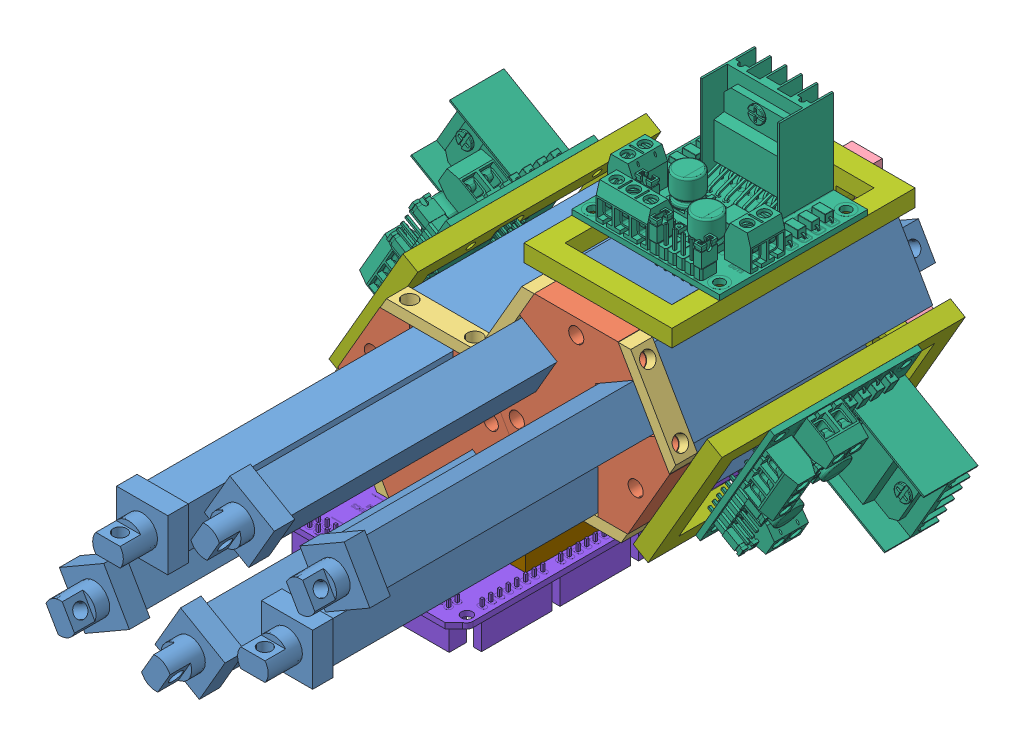
SolidWorks assembly DeltaArray, configuration Default. Lengths in mm.
Overall size (160.54 122.18 184.94).
31 component instances, 9 part files, 18 mates.
Components (placement in the parent):
- Delta_Module-1: Delta_Module [Default] at (-24.2565 17.4629 11.2137) size (68.32 71 180)
  - 3inLinearActuator-1: 3inLinearActuator [Default] at (52.9296 100.0903 59.6287) size (23 19 180)
  - 3inLinearActuator-2: 3inLinearActuator [Default] at (66.3243 77.8201 59.6287) x (-0.5 -0.866025 0) z (0 0 1) size (23 19 180)
  - 3inLinearActuator-3: 3inLinearActuator [Default] at (40.3403 77.3551 59.6287) x (-0.5 0.866025 0) z (0 0 1) size (23 19 180)
  - Connector-1: Connector [Default] at (53.1981 85.0885 129.6287) x (-0.5 0.866025 0) z (0.866025 0.5 0) size (54.66 6.35 47.33)
  - Edge_Piece-1: Edge_Piece [Default] at (53.1981 107.9385 129.6287) x (-1 0 0) z (0 0 1) size (29.97 3.17 6.35)
  - Edge_Piece-2: Edge_Piece [Default] at (33.4094 73.6635 129.6287) x (0.5 -0.866025 0) z (0 0 1) size (29.97 3.17 6.35)
  - Edge_Piece-3: Edge_Piece [Default] at (72.9867 73.6635 129.6287) x (0.5 0.866025 0) z (0 0 1) size (29.97 3.17 6.35)
  - BottomConnector-1: BottomConnector [Default] at (53.1981 85.0885 58.4387) x (0.5 -0.866025 0) z (0.866025 0.5 0) size (46.87 7.62 40.59)
- Delta_Module-2: Delta_Module [Default] at (118.44 38.4209 11.2137) x (0.5 0.866025 0) z (0 0 1) size (68.32 71 180)
  - 3inLinearActuator-1: 3inLinearActuator [Default] at (52.9296 100.0903 59.6287) size (23 19 180)
  - 3inLinearActuator-2: 3inLinearActuator [Default] at (66.3243 77.8201 59.6287) x (-0.5 -0.866025 0) z (0 0 1) size (23 19 180)
  - 3inLinearActuator-3: 3inLinearActuator [Default] at (40.3403 77.3551 59.6287) x (-0.5 0.866025 0) z (0 0 1) size (23 19 180)
  - Connector-1: Connector [Default] at (53.1981 85.0885 129.6287) x (-0.5 0.866025 0) z (0.866025 0.5 0) size (54.66 6.35 47.33)
  - Edge_Piece-1: Edge_Piece [Default] at (53.1981 107.9385 129.6287) x (-1 0 0) z (0 0 1) size (29.97 3.17 6.35)
  - Edge_Piece-2: Edge_Piece [Default] at (33.4094 73.6635 129.6287) x (0.5 -0.866025 0) z (0 0 1) size (29.97 3.17 6.35)
  - Edge_Piece-3: Edge_Piece [Default] at (72.9867 73.6635 129.6287) x (0.5 0.866025 0) z (0 0 1) size (29.97 3.17 6.35)
  - BottomConnector-1: BottomConnector [Default] at (53.1981 85.0885 58.4387) x (0.5 -0.866025 0) z (0.866025 0.5 0) size (46.87 7.62 40.59)
- Franka_Delta_Mount-1: Franka_Delta_Mount [Default] at (50.1459 114.7937 57.2699) x (0.866025 0.5 0) z (0 0 1) size (61 61 4.76)
- L298N_Assembly-1: L298N_Assembly [Default] at (78.5597 116.9066 58.7944) x (-0.499999 -0.866024 0.00149) z (0.000745 0.00129 0.999999) size (43.41 40 71.25)
  - L298N Dual H Bridge-1: L298N Dual H Bridge [Default] at (-5.0709 19.6717 46.4281) size (43.3 28.21 43.3)
  - L298NHolder-1: L298NHolder [Default] at (-5.0983 18.1317 46.4607) x (-0.999999 0 0.00149) z (0 -1 0) size (43.3 71.19 13.8)
- L298N_Assembly-2: L298N_Assembly [Default] at (76.5177 138.3444 58.7944) x (0.999999 0 0.00149) z (-0.00149 0 0.999999) size (43.41 40 71.25)
  - L298N Dual H Bridge-1: L298N Dual H Bridge [Default] at (-5.0709 19.6717 46.4281) size (43.3 28.21 43.3)
  - L298NHolder-1: L298NHolder [Default] at (-5.0983 18.1317 46.4607) x (-0.999999 0 0.00149) z (0 -1 0) size (43.3 71.19 13.8)
- L298N_Assembly-3: L298N_Assembly [Default] at (21.732 112.6807 58.7944) x (0.499999 0.866024 0.00149) z (-0.000745 -0.00129 0.999999) size (43.41 40 71.25)
  - L298N Dual H Bridge-1: L298N Dual H Bridge [Default] at (-5.0709 19.6717 46.4281) size (43.3 28.21 43.3)
  - L298NHolder-1: L298NHolder [Default] at (-5.0983 18.1317 46.4607) x (-0.999999 0 0.00149) z (0 -1 0) size (43.3 71.19 13.8)
- ArduinoMegaAssembly-1: ArduinoMegaAssembly [Default] at (43.5719 128.8662 18.719) x (-1 0 0) z (0 0 1) size (53.6 26.41 108.35)
  - Arduino MEGA 2560 R3-1: Arduino MEGA 2560 R3 [Default] at (15.5804 57.3596 95.7334) size (53.6 14.61 108.35)
  - ArduinoMegaHolder-1: ArduinoMegaHolder [Default] at (14.6304 55.7596 86.5284) x (1 0 0) z (0 -1 0) size (38.5 71.19 13.8)
Mates (geometry in assembly coordinates):
- Coincident1: coincident anti-aligned: plane of Delta_Module-1/Connector-1 through (50.1459 114.7937 147.1924) normal (0.866025 0.5 0); plane of Delta_Module-2/Connector-1 through (50.1459 114.7937 147.1924) normal (-0.866025 -0.5 0)
- Coincident2: coincident aligned: plane of Delta_Module-1/Connector-1 through (28.9415 102.5514 147.1924) normal (0 0 1); plane of Delta_Module-2/Connector-1 through (71.3502 127.036 147.1924) normal (0 0 1)
- Width1: width anti-aligned: plane of Delta_Module-1/BottomConnector-1 through (26.719 106.4008 62.0324) normal (-0.5 0.866025 0); plane of Delta_Module-1/BottomConnector-1 through (31.164 98.7019 62.0324) normal (0.5 -0.866025 0); plane of Delta_Module-2/BottomConnector-1 through (73.5727 123.1865 62.0324) normal (0.5 -0.866025 0); plane of Delta_Module-2/BottomConnector-1 through (69.1277 130.8855 62.0324) normal (-0.5 0.866025 0)
- Coincident5: coincident anti-aligned: plane of Delta_Module-1/BottomConnector-1 through (28.9415 102.5514 62.0324) normal (0 0 -1); plane of Franka_Delta_Mount-1 through (50.1459 114.7937 62.0324) normal (0 0 1)
- Width5: width anti-aligned: plane of Delta_Module-1/3inLinearActuator-3 through (14.1427 88.2337 61.8424) normal (0.5 -0.866025 0); plane of Delta_Module-1/3inLinearActuator-3 through (9.1427 96.894 61.8424) normal (-0.5 0.866025 0); plane of Franka_Delta_Mount-1 through (47.6059 119.1931 62.0324) normal (-0.5 0.866025 0); plane of Franka_Delta_Mount-1 through (52.6859 110.3943 62.0324) normal (0.5 -0.866025 0)
- Width6: width anti-aligned: plane of Delta_Module-1/3inLinearActuator-3 through (9.1427 96.894 61.8424) normal (-0.866025 -0.5 0); plane of Delta_Module-2/3inLinearActuator-2 through (91.1491 132.6934 61.8424) normal (0.866025 0.5 0); plane of Franka_Delta_Mount-1 through (76.5596 130.0437 62.0324) normal (0.866025 0.5 0); plane of Franka_Delta_Mount-1 through (23.7321 99.5437 62.0324) normal (-0.866025 -0.5 0)
- Concentric4: concentric aligned: cylinder of Delta_Module-2/Connector-1 through (88.7445 116.9934 147.1924) axis (0 0 -1) radius 2.2225; cylinder of L298N_Assembly-1/L298NHolder-1 through (88.7445 116.9934 140.8424) axis (0 0 -1) radius 2.2479
- Parallel1: parallel anti-aligned: plane of Delta_Module-2/Connector-1 through (92.5545 114.7937 147.1924) normal (0.866025 -0.5 0); plane of L298N_Assembly-1/L298NHolder-1 through (92.5159 114.816 105.2474) normal (-0.866025 0.5 0)
- Coincident17: coincident anti-aligned: plane of Delta_Module-2/Connector-1 through (71.3502 127.036 140.8424) normal (0 0 -1); plane of L298N_Assembly-1/L298NHolder-1 through (81.6909 96.0666 140.8424) normal (0 0 1)
- Concentric5: concentric anti-aligned: circle of Delta_Module-2/Connector-1; circle of L298N_Assembly-2/L298NHolder-1
- Coincident18: coincident anti-aligned: plane of Delta_Module-2/Connector-1 through (71.3502 127.036 140.8424) normal (0 0 -1); plane of L298N_Assembly-2/L298NHolder-1 through (93.0002 151.476 140.8424) normal (0 0 1)
- Parallel2: parallel anti-aligned: plane of Delta_Module-2/Connector-1 through (71.3502 151.5207 147.1924) normal (0 1 0); plane of L298N_Assembly-2/L298NHolder-1 through (71.3502 151.476 105.2474) normal (0 -1 0)
- Concentric6: concentric aligned: cylinder of Delta_Module-1/Connector-1 through (11.5472 112.594 147.1924) axis (0 0 -1) radius 2.2225; circle of L298N_Assembly-3/L298NHolder-1
- Coincident20: coincident anti-aligned: plane of Delta_Module-1/Connector-1 through (28.9415 102.5514 140.8424) normal (0 0 -1); plane of L298N_Assembly-3/L298NHolder-1 through (18.6008 133.5208 140.8424) normal (0 0 1)
- Parallel3: parallel anti-aligned: plane of Delta_Module-1/Connector-1 through (7.7372 114.7937 147.1924) normal (-0.866025 0.5 0); plane of L298N_Assembly-3/L298NHolder-1 through (7.7758 114.7714 105.2474) normal (0.866025 -0.5 0)
- Concentric8: concentric aligned: circle of Delta_Module-1/BottomConnector-1; circle of ArduinoMegaAssembly-1/ArduinoMegaHolder-1
- Coincident29: coincident anti-aligned: plane of Delta_Module-1/Connector-1 through (28.9415 102.5514 140.8424) normal (0 0 -1); plane of ArduinoMegaAssembly-1/ArduinoMegaHolder-1 through (50.5915 78.1066 140.8424) normal (0 0 1)
- Parallel7: parallel anti-aligned: plane of Delta_Module-1/Connector-1 through (28.9415 78.0667 147.1924) normal (0 -1 0); plane of ArduinoMegaAssembly-1/ArduinoMegaHolder-1 through (28.9415 78.1066 105.2474) normal (0 1 0)
